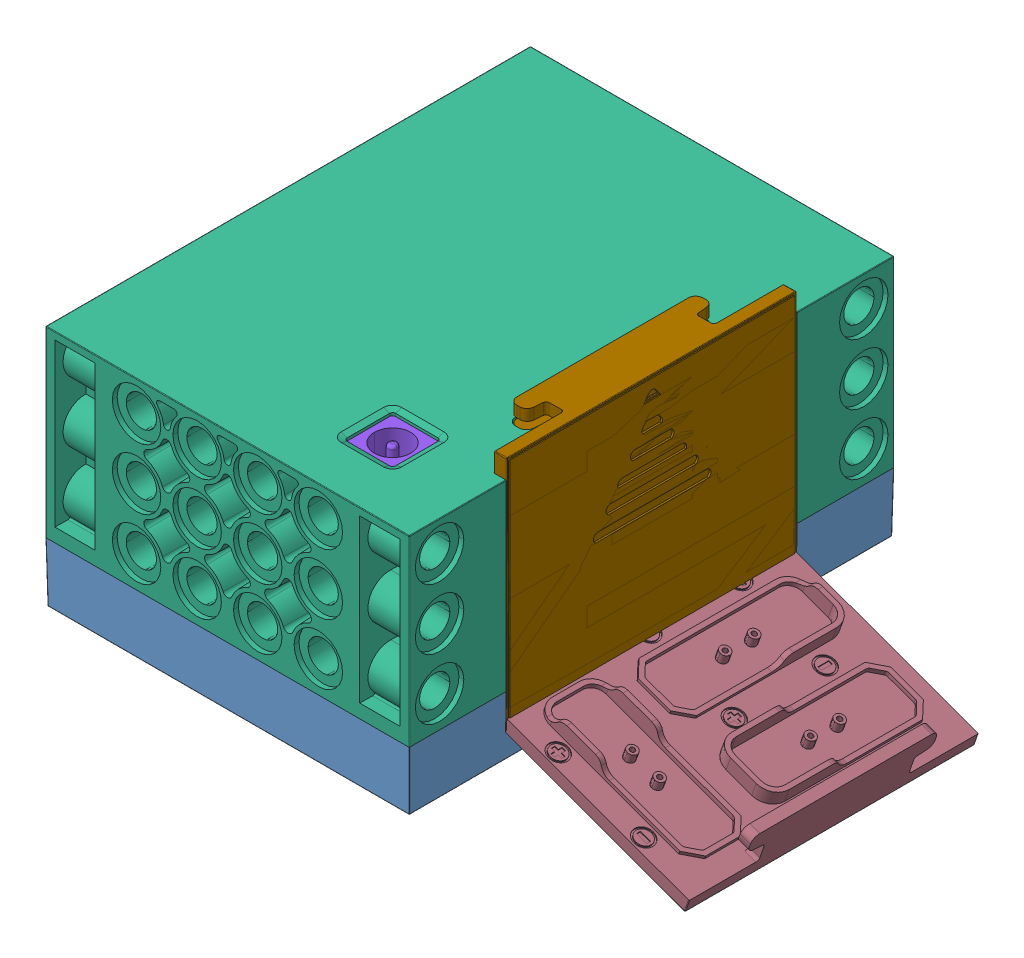
SolidWorks assembly babeta-20220407, configuration Default. Lengths in mm.
Overall size (92.17 50.21 80.41).
26 component instances, 15 part files, 0 mates.
Components (placement in the parent):
- babeta-20220407(2)^babeta-20220407-1: babeta-20220407(2)^babeta-20220407 [Default] at origin size (92.17 50.21 80.41) (virtual)
  - BABETA_V2_ANY_ASM^babeta-20220407(2)_babeta-20220407-1: BABETA_V2_ANY_ASM^babeta-20220407(2)_babeta-20220407 [Default] at origin size (60.1 43.06 80.41) (virtual)
    - BACA_BOTTOM_ANY_ASM^BABETA_V2_ANY_ASM_babeta-20220407(2)_babeta-20220407-1: BACA_BOTTOM_ANY_ASM^BABETA_V2_ANY_ASM_babeta-20220407(2)_babeta-20220407 [Default] at origin size (60.01 38.31 80.01) (virtual)
      - BOSS-EXTRUDE5^BACA_BOTTOM_ANY_ASM_BABETA_V2_ANY_ASM_babeta-20220407(2)_babeta-20220407-1: BOSS-EXTRUDE5^BACA_BOTTOM_ANY_ASM_BABETA_V2_ANY_ASM_babeta-20220407(2)_babeta-20220407 [Default] at origin size (60.01 38.31 80.01) (virtual)
      - CUT-EXTRUDE3_3_^BACA_BOTTOM_ANY_ASM_BABETA_V2_ANY_ASM_babeta-20220407(2)_babeta-20220407-1: CUT-EXTRUDE3_3_^BACA_BOTTOM_ANY_ASM_BABETA_V2_ANY_ASM_babeta-20220407(2)_babeta-20220407 [Default] at origin size (0.06 0.4 6.95) (virtual)
      - CUT-EXTRUDE3_2_^BACA_BOTTOM_ANY_ASM_BABETA_V2_ANY_ASM_babeta-20220407(2)_babeta-20220407-1: CUT-EXTRUDE3_2_^BACA_BOTTOM_ANY_ASM_BABETA_V2_ANY_ASM_babeta-20220407(2)_babeta-20220407 [Default] at origin size (0.06 0.4 6.95) (virtual)
      - CUT-EXTRUDE3_4_^BACA_BOTTOM_ANY_ASM_BABETA_V2_ANY_ASM_babeta-20220407(2)_babeta-20220407-1: CUT-EXTRUDE3_4_^BACA_BOTTOM_ANY_ASM_BABETA_V2_ANY_ASM_babeta-20220407(2)_babeta-20220407 [Default] at origin size (0.06 0.4 6.95) (virtual)
      - CUT-EXTRUDE3_5_^BACA_BOTTOM_ANY_ASM_BABETA_V2_ANY_ASM_babeta-20220407(2)_babeta-20220407-1: CUT-EXTRUDE3_5_^BACA_BOTTOM_ANY_ASM_BABETA_V2_ANY_ASM_babeta-20220407(2)_babeta-20220407 [Default] at origin size (0.06 0.4 6.95) (virtual)
    - BACA_TOP_ANY^BABETA_V2_ANY_ASM_babeta-20220407(2)_babeta-20220407-1: BACA_TOP_ANY^BABETA_V2_ANY_ASM_babeta-20220407(2)_babeta-20220407 [Default] at origin size (60.01 31.6 80.41) (virtual)
    - BA_BATTERY_ANY^BABETA_V2_ANY_ASM_babeta-20220407(2)_babeta-20220407-1: BA_BATTERY_ANY^BABETA_V2_ANY_ASM_babeta-20220407(2)_babeta-20220407 [Default] at (-112.9 29.95 15) x (0 1 0) z (1 0 0) size (14.5 14.5 50.5) (virtual)
    - BA_BATTERY_ANY^BABETA_V2_ANY_ASM_babeta-20220407(2)_babeta-20220407-2: BA_BATTERY_ANY^BABETA_V2_ANY_ASM_babeta-20220407(2)_babeta-20220407 [Default] at (-65.4 29.95 0) x (0 -1 0) z (-1 0 0) size (14.5 14.5 50.5) (virtual)
    - BA_BATTERY_ANY^BABETA_V2_ANY_ASM_babeta-20220407(2)_babeta-20220407-3: BA_BATTERY_ANY^BABETA_V2_ANY_ASM_babeta-20220407(2)_babeta-20220407 [Default] at (-65.4 14.95 15) x (0 -1 0) z (-1 0 0) size (14.5 14.5 50.5) (virtual)
    - BA_BATTERY_ANY^BABETA_V2_ANY_ASM_babeta-20220407(2)_babeta-20220407-4: BA_BATTERY_ANY^BABETA_V2_ANY_ASM_babeta-20220407(2)_babeta-20220407 [Default] at (-65.4 14.95 -15) x (0 -1 0) z (-1 0 0) size (14.5 14.5 50.5) (virtual)
    - PART2_BABETA_V2_ANY^BABETA_V2_ANY_ASM_babeta-20220407(2)_babeta-20220407-1: PART2_BABETA_V2_ANY^BABETA_V2_ANY_ASM_babeta-20220407(2)_babeta-20220407 [Default] at (-0.5 39.2 -1.6) x (1 0 0) z (0 1 0) size (9 9 10) (virtual)
    - BA_BATTERY_ANY^BABETA_V2_ANY_ASM_babeta-20220407(2)_babeta-20220407-5: BA_BATTERY_ANY^BABETA_V2_ANY_ASM_babeta-20220407(2)_babeta-20220407 [Default] at (-112.9 14.95 0) x (0 1 0) z (1 0 0) size (14.5 14.5 50.5) (virtual)
    - BA_BATTERY_ANY^BABETA_V2_ANY_ASM_babeta-20220407(2)_babeta-20220407-6: BA_BATTERY_ANY^BABETA_V2_ANY_ASM_babeta-20220407(2)_babeta-20220407 [Default] at (-112.9 29.95 -15) x (0 1 0) z (1 0 0) size (14.5 14.5 50.5) (virtual)
    - PART1_BABETA_V2_ANY^BABETA_V2_ANY_ASM_babeta-20220407(2)_babeta-20220407-1: PART1_BABETA_V2_ANY^BABETA_V2_ANY_ASM_babeta-20220407(2)_babeta-20220407 [Default] at (-60 0 0) x (0 0 -1) z (1 0 0) size (49.6 36.35 8.22) (virtual)
    - PART1_BABETA_V2_ANY^BABETA_V2_ANY_ASM_babeta-20220407(2)_babeta-20220407-2: PART1_BABETA_V2_ANY^BABETA_V2_ANY_ASM_babeta-20220407(2)_babeta-20220407 [Default] at (-60 3.1 0) x (0 0 -1) z (1 0 0) size (49.6 36.35 8.22) (virtual)
    - TAN-PIAN^BABETA_V2_ANY_ASM_babeta-20220407(2)_babeta-20220407-1: TAN-PIAN^BABETA_V2_ANY_ASM_babeta-20220407(2)_babeta-20220407 [Default] at origin size (9.33 23 8) (virtual)
    - TAN-PIAN-A^BABETA_V2_ANY_ASM_babeta-20220407(2)_babeta-20220407-1: TAN-PIAN-A^BABETA_V2_ANY_ASM_babeta-20220407(2)_babeta-20220407 [Default] at (0 59.8738 -0.0522) x (1 0 0) z (0 -0.001745 -0.999998) size (9.15 8.02 15.93) (virtual)
    - TAN-PIAN-A^BABETA_V2_ANY_ASM_babeta-20220407(2)_babeta-20220407-2: TAN-PIAN-A^BABETA_V2_ANY_ASM_babeta-20220407(2)_babeta-20220407 [Default] at (0 45.88 -29.4659) x (1 0 0) z (0 -0.573576 -0.819152) size (9.15 8.02 15.93) (virtual)
    - TAN-PIAN-B^BABETA_V2_ANY_ASM_babeta-20220407(2)_babeta-20220407-1: TAN-PIAN-B^BABETA_V2_ANY_ASM_babeta-20220407(2)_babeta-20220407 [Default] at origin size (2.02 8.3 25.8) (virtual)
  - PART1_BABETA_V2_ANY^babeta-20220407(2)_babeta-20220407-1: PART1_BABETA_V2_ANY^babeta-20220407(2)_babeta-20220407 [Default] at (-68.1608 6.5858 0) x (0 0 -1) z (-0.34202 -0.939693 0) size (49.6 36.35 8.22) (virtual)
  - TAN-PIAN^babeta-20220407(2)_babeta-20220407-1: TAN-PIAN^babeta-20220407(2)_babeta-20220407 [Default] at (0 29.95 29.95) x (1 0 0) z (0 1 0) size (9.33 23 8) (virtual)
  - TAN-PIAN-B^babeta-20220407(2)_babeta-20220407-1: TAN-PIAN-B^babeta-20220407(2)_babeta-20220407 [Default] at (0 44.9 -15) x (1 0 0) z (0 0 -1) size (2.02 8.3 25.8) (virtual)
  - TAN-PIAN-B^babeta-20220407(2)_babeta-20220407-2: TAN-PIAN-B^babeta-20220407(2)_babeta-20220407 [Default] at (0 29.95 29.95) x (1 0 0) z (0 1 0) size (2.02 8.3 25.8) (virtual)
